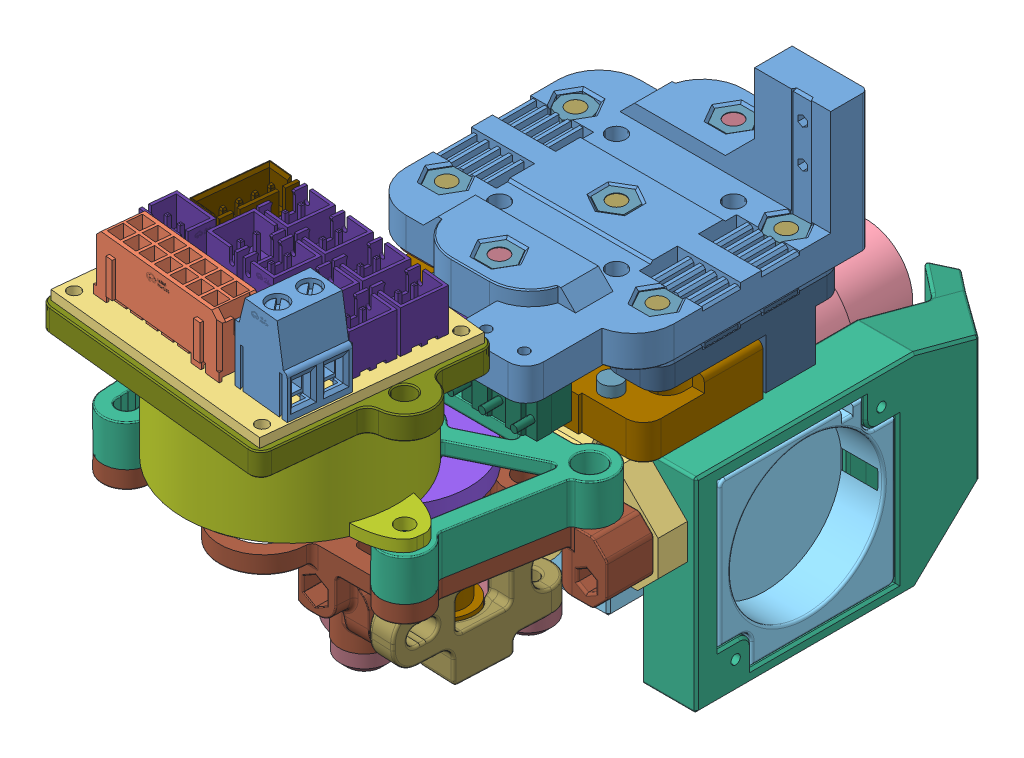
SolidWorks assembly TAP+换头组装, configuration 默认. Lengths in mm.
Overall size (64.42 74.4 119.93).
93 component instances, 36 part files, 59 mates.
Components (placement in the parent):
- TAP+换头-底座-1: TAP+换头-底座 [默认] at (-24.6795 -3.9341 35) size (46 23.5 58)
- MGN9H v1 v1-1: MGN9H v1 v1 [默认] at (-185.6361 139.1341 -146.0548) x (0 -1 0) z (-1 0 0) size (8 40.67 20)
- TAP+换头-热端装配-1: TAP+换头-热端装配 [默认] at (-3.9804 -84.1007 64.8164) x (-1 0 0) z (0 1 0) size (64.42 119.93 74.4)
  - TAP+换头-V6固定座-1: TAP+换头-V6固定座 [Default] at (0.6992 -1.423 53.775) size (52 19.4 22.55)
  - V6散热器-1: V6散热器 [Default] at (0.6992 1.577 53.775) x (-0.937959 0 -0.346747) z (-0.346747 0 0.937959) size (22.3 59 22.3)
  - TAP+换头-V6固定座-1-1: TAP+换头-V6固定座-1 [Default] at (0.6992 -1.423 53.775) x (-1 0 0) z (0 0 -1) size (35 25.4 12.09)
  - 挤出机组装-1: 挤出机组装 [Default] at (24.2197 76.008 94.8824) x (-1 0 0) z (0 -1 0) size (60.01 46.35 49.65)
    - 挤出机电机座-1: 挤出机电机座 [Default] at (-24.1653 27.1074 25.8748) size (56.72 7.01 44.47)
    - 36圆饼电机-1: 36圆饼电机 [Default] at (15.4671 9.6074 38.1257) x (0.994716 0 -0.102664) z (0.102664 0 0.994716) size (49.93 29 36.4)
    - BMG主齿组装-1: BMG主齿组装 [Default] at (16.3112 26.812 26.7681) x (0.995449 0 0.095298) z (-0.095298 0 0.995449) size (25.9 28.3 25.9)
      - BMG主齿-1: BMG主齿 [Default] at (5.4147 0.2954 24.6592) size (25.9 28.3 25.9)
      - BMG挤出齿-1: BMG挤出齿 [Default] at (5.4147 25.5954 24.6592) x (-0.887226 0 -0.461335) z (-0.461335 0 0.887226) size (9.4 14 9.4)
    - MR85-1: MR85 [Default] at (19.3513 27.6074 51.831) size (8 2.5 8)
    - 挤出机主体-1: 挤出机主体 [Default] at (-24.1653 34.1074 25.8748) size (59.44 18.3 40.97)
    - 挤出机从挤出齿轮支架-1: 挤出机从挤出齿轮支架 [Default] at (34.3823 55.9074 36.7653) x (0.043131 0 0.999069) z (0 -1 0) size (30 8.53 21.09)
    - BMG挤出齿-2: BMG挤出齿 [Default] at (28.0327 52.4074 51.9833) x (-0.837169 0 -0.546944) z (-0.546944 0 0.837169) size (9.4 14 9.4)
    - 挤出机盖子-1: 挤出机盖子 [Default] at (19.3513 55.9074 51.831) x (0.999977 0 0.006798) z (0.006798 0 -0.999977) size (25.23 3.5 27.46)
    - MR85-2: MR85 [Default] at (19.3513 54.9074 51.831) x (-0.837169 0 -0.546944) z (-0.546944 0 0.837169) size (8 2.5 8)
  - M3螺母-1: M3螺母 [默认] at (12.1907 1.0199 62.875) x (-0.783317 0.621622 0) z (0.621622 0.783317 0) size (6.35 2.3 5.5)
  - M3x20-1: M3x20 [Default] at (12.1992 1.077 65.275) x (-0.825766 -0.564012 0) z (0 0 -1) size (5.7 5.7 23)
  - M3螺母-2: M3螺母 [默认] at (-10.8461 1.0411 62.875) x (-0.929999 0.367561 0) z (0.367561 0.929999 0) size (6.35 2.3 5.5)
  - M3x20-2: M3x20 [Default] at (-10.8461 1.0411 65.275) x (-0.518434 0.855118 0) z (0 0 -1) size (5.7 5.7 23)
  - PCB固定-2-2: PCB固定-2 [默认] at (-13.6764 25.1175 89.275) x (0.102664 0.994716 0) z (-0.994716 0.102664 0) size (37 4 53.35)
  - 3D_HeadBoard_2024-03-10.step-1: 3D_HeadBoard_2024-03-10.step [默认] at (-8.9858 60.8247 89.275) x (0.994716 -0.102664 0) z (0 0 1) size (39.97 34.97 17.5)
    - FAN2.step-1: FAN2.step [默认] at (13.0535 -19.558 1.6001) x (0 -1 0) z (0 0 1) size (7.5 5.9 10.6)
      - CONN-TH_2P-P2.50_HX25003-2A.step-1: CONN-TH_2P-P2.50_HX25003-2A.step [默认] at origin size (7.5 5.9 10.6)
        - COMPOUND.step-1: COMPOUND.step [默认] at origin size (7.5 5.9 10.6)
    - PROBE.step-1: PROBE.step [默认] at (13.0535 -27.5591 1.6001) x (0 -1 0) z (0 0 1) size (7.5 5.9 10.6)
      - CONN-TH_2P-P2.50_HX25003-2A.step-1: CONN-TH_2P-P2.50_HX25003-2A.step [默认] at origin size (7.5 5.9 10.6)
        - COMPOUND.step-1: COMPOUND.step [默认] at origin size (7.5 5.9 10.6)
    - TEM1.step-1: TEM1.step [默认] at (27.4766 -27.5591 1.6001) x (0 -1 0) z (0 0 1) size (7.5 5.9 10.6)
      - CONN-TH_2P-P2.50_HX25003-2A.step-1: CONN-TH_2P-P2.50_HX25003-2A.step [默认] at origin size (7.5 5.9 10.6)
        - COMPOUND.step-1: COMPOUND.step [默认] at origin size (7.5 5.9 10.6)
    - TEM2.step-1: TEM2.step [默认] at (20.2651 -27.5591 1.6001) x (0 -1 0) z (0 0 1) size (7.5 5.9 10.6)
      - CONN-TH_2P-P2.50_HX25003-2A.step-1: CONN-TH_2P-P2.50_HX25003-2A.step [默认] at origin size (7.5 5.9 10.6)
        - COMPOUND.step-1: COMPOUND.step [默认] at origin size (7.5 5.9 10.6)
    - 5V.step-1: 5V.step [默认] at (34.6711 -14.859 1.6001) size (7.5 5.9 10.6)
      - CONN-TH_2P-P2.50_HX25003-2A.step-1: CONN-TH_2P-P2.50_HX25003-2A.step [默认] at origin size (7.5 5.9 10.6)
        - COMPOUND.step-1: COMPOUND.step [默认] at origin size (7.5 5.9 10.6)
    - FAN2-1.step-1: FAN2-1.step [默认] at (5.842 -19.558 1.6001) x (0 -1 0) z (0 0 1) size (7.5 5.9 10.6)
      - CONN-TH_2P-P2.50_HX25003-2A.step-1: CONN-TH_2P-P2.50_HX25003-2A.step [默认] at origin size (7.5 5.9 10.6)
        - COMPOUND.step-1: COMPOUND.step [默认] at origin size (7.5 5.9 10.6)
    - X-ENDSTOP.step-1: X-ENDSTOP.step [默认] at (5.842 -27.5591 1.6001) x (0 -1 0) z (0 0 1) size (7.5 5.9 10.6)
      - CONN-TH_2P-P2.50_HX25003-2A.step-1: CONN-TH_2P-P2.50_HX25003-2A.step [默认] at origin size (7.5 5.9 10.6)
        - COMPOUND.step-1: COMPOUND.step [默认] at origin size (7.5 5.9 10.6)
    - VCC.step-1: VCC.step [默认] at (26.1621 -19.558 1.6001) x (0 1 0) z (0 0 1) size (7.5 5.9 10.6)
      - CONN-TH_2P-P2.50_HX25003-2A.step-1: CONN-TH_2P-P2.50_HX25003-2A.step [默认] at origin size (7.5 5.9 10.6)
        - COMPOUND.step-1: COMPOUND.step [默认] at origin size (7.5 5.9 10.6)
    - FAN1.step-1: FAN1.step [默认] at (20.2651 -19.558 1.6001) x (0 -1 0) z (0 0 1) size (7.5 5.9 10.6)
      - CONN-TH_2P-P2.50_HX25003-2A.step-1: CONN-TH_2P-P2.50_HX25003-2A.step [默认] at origin size (7.5 5.9 10.6)
        - COMPOUND.step-1: COMPOUND.step [默认] at origin size (7.5 5.9 10.6)
    - E_MOTO.step-1: E_MOTO.step [默认] at (33.2741 -25.0864 1.6001) x (0 -1 0) z (0 0 1) size (12.5 5.7 10)
      - CONN-TH_4P-P2.50_4PIN.step-1: CONN-TH_4P-P2.50_4PIN.step [默认] at origin size (12.5 5.7 10)
        - COMPOUND-0.step-1: COMPOUND-0.step [默认] at origin size (12.5 5.7 10)
    - HOT.step-1: HOT.step [默认] at (5.842 -9.652 1.6001) x (0 1 0) z (0 0 1) size (10.76 10 17.5)
      - CONN-TH_2P-P5.00_WJ500V-5.08-2P.step-1: CONN-TH_2P-P5.00_WJ500V-5.08-2P.step [默认] at origin size (10.76 10 17.5)
        - COMPOUND-1.step-1: COMPOUND-1.step [默认] at origin size (10.76 10 17.5)
    - HEAD_IN.step-1: HEAD_IN.step [默认] at (24.003 -6.858 1.6001) x (-1 0 0) z (0 0 1) size (24 8.8 13.2)
      - CONN-TH_14P-P3.00_HC-MX3.0-2X7A.step-1: CONN-TH_14P-P3.00_HC-MX3.0-2X7A.step [默认] at origin size (24 8.8 13.2)
        - SOLID.step-1: SOLID.step [默认] at origin size (24 8.8 13.2)
    - COMPOUND-2.step-1: COMPOUND-2.step [默认] at origin size (39.97 34.97 1.6)
  - 3010风扇-1: 3010风扇 [Default] at (-14.3008 -39.823 42.275) x (1 0 0) z (0 1 0) size (30 10 30)
  - 3010涡轮-1: 3010涡轮 [Default] at (-16.8008 0.077 32.875) x (0 0 1) z (0 -1 0) size (30 10.07 30)
  - V2吹料-1-1: V2吹料-1 [默认] at (-26.8008 0.077 65.275) size (16.15 60.54 34.8)
  - 镜向V2吹料-1-2: 镜向V2吹料-1 [默认] at (28.1992 0.077 65.275) x (-1 0 0) z (0 0 -1) size (16.15 60.54 34.8)
  - 3010涡轮-2: 3010涡轮 [Default] at (18.1992 0.077 62.875) x (0 0 -1) z (0 -1 0) size (30 10.07 30)
- MGN9-6-1: MGN9-6 [默认] at (-4.6795 -6.5841 292.5) x (1 0 0) z (0 0 -1) size (9 6.5 50)
- TAP+换头中间座-1: TAP+换头中间座 [默认] at (-17.1795 -17.3341 73.9934) size (46 8.6 30)
- TAP+换头皮带盖板-2: TAP+换头皮带盖板 [默认] at (8.3205 -7.9341 71) size (10 12.6 32)
- TAP+换头皮带盖板-2-1: TAP+换头皮带盖板-2 [默认] at (-27.6795 -7.9341 71) size (10 12.6 32)
- M3x8-1: M3x8 [Default] at (-22.6795 1.0659 66) x (0.99943 0 -0.033759) z (0 -1 0) size (5.7 5.7 11)
- M3x8-2: M3x8 [Default] at (-22.6795 1.0659 44) x (0.753968 0 0.656911) z (0 -1 0) size (5.7 5.7 11)
- M3x8-4: M3x8 [Default] at (13.3205 1.0659 66) x (0.058047 0 -0.998314) z (0 -1 0) size (5.7 5.7 11)
- M3x8-5: M3x8 [Default] at (13.3205 1.0659 44) x (0.586032 0 0.810288) z (0 -1 0) size (5.7 5.7 11)
- M3x8-7: M3x8 [Default] at (-4.6795 1.6659 54.992) x (-0.906074 0 -0.423119) z (0 -1 0) size (5.7 5.7 11)
- M3螺母-2: M3螺母 [默认] at (13.3205 -1.2341 66) x (0.512033 0 -0.858966) z (0.858966 0 0.512033) size (6.35 2.3 5.5)
- M3螺母-3: M3螺母 [默认] at (-4.6795 -0.5341 55) x (-0.011209 0 -0.999937) z (0.999937 0 -0.011209) size (6.35 2.3 5.5)
- M3螺母-4: M3螺母 [默认] at (-4.6795 1.4659 75) size (6.35 2.3 5.5)
- M3x10-2: M3x10 [Default] at (-4.6795 3.6659 75) x (-0.258789 0 0.965934) z (0 -1 0) size (5.7 5.7 13)
- M3螺母-5: M3螺母 [默认] at (-4.6795 1.4659 35) size (6.35 2.3 5.5)
- M3x10-3: M3x10 [Default] at (-4.6795 3.6659 35) x (-0.379423 0 -0.925223) z (0 -1 0) size (5.7 5.7 13)
- M3螺母-6: M3螺母 [默认] at (13.3205 -1.2341 44) x (0.999299 0 -0.037424) z (0.037424 0 0.999299) size (6.35 2.3 5.5)
- M3螺母-7: M3螺母 [默认] at (-22.6795 -1.2341 66) size (6.35 2.3 5.5)
- M3螺母-8: M3螺母 [默认] at (-22.6795 -1.2341 44) x (0.719334 0 -0.694664) z (0.694664 0 0.719334) size (6.35 2.3 5.5)
- M2x8-1: M2x8 [Default] at (-17.1795 -18.2341 58.9934) x (-0.826538 0 -0.562881) z (0 1 0) size (3.6 3.6 9.8)
- M2x8-2: M2x8 [Default] at (7.8205 -18.2341 58.9934) x (1 0 0) z (0 1 0) size (3.6 3.6 9.8)
- M2x8-3: M2x8 [Default] at (9.8205 -19.3341 70.3934) x (-0.826538 0 -0.562881) z (0 1 0) size (3.6 3.6 9.8)
- M2x8-4: M2x8 [Default] at (-19.1795 -19.3341 70.3934) x (-0.826538 0 -0.562881) z (0 1 0) size (3.6 3.6 9.8)
- KW10 Microswitch v1-1: KW10 Microswitch v1 [默认] at (86.3205 84.1659 86.4) x (1 0 0) z (0 0 -1) size (13.18 11.3 12.93)
  - M2x10 Self-tapping Screw (14) v1^KW10 Microswitch v1-1: M2x10 Self-tapping Screw (14) v1^KW10 Microswitch v1 [默认] at (-76.75 95.2 1.4) x (0 0 1) z (0 1 0) size (3.5 3.5 11.3) (hidden, virtual)
  - M2x10 Self-tapping Screw (14) v1 (1)^KW10 Microswitch v1-1: M2x10 Self-tapping Screw (14) v1 (1)^KW10 Microswitch v1 [默认] at (-83.25 95.2 1.4) x (0 0 1) z (0 1 0) size (3.5 3.5 11.3) (hidden, virtual)
  - KW10 Microswitch v1-3^KW10 Microswitch v1-1: KW10 Microswitch v1-3^KW10 Microswitch v1 [默认] at origin size (13.08 3.8 4.39) (hidden, virtual)
  - KW10 Microswitch v1-4^KW10 Microswitch v1-1: KW10 Microswitch v1-4^KW10 Microswitch v1 [默认] at origin size (12.8 5.8 10.15) (virtual)
Mates (geometry in assembly coordinates):
- 重合4: coincident anti-aligned: plane of MGN9H v1 v1-1 through (-4.6795 -9.8341 73.9434) normal (0 1 0); plane of MGN9-6-1 through (-8.9795 -9.8341 42.5) normal (0 -1 0)
- 重合5: coincident anti-aligned: plane of MGN9H v1 v1-1 through (-9.1795 -9.3341 73.9434) normal (1 0 0); plane of MGN9-6-1 through (-9.1795 -3.5341 42.5) normal (-1 0 0)
- 同心9: concentric aligned: cylinder of MGN9H v1 v1-1 through (2.8205 -10.3341 50.9934) axis (0 -1 0) radius 1.5; cylinder of TAP+换头中间座-1 through (2.8205 -13.3341 50.9934) axis (0 -1 0) radius 1.6
- 同心10: concentric aligned: cylinder of MGN9H v1 v1-1 through (-12.1795 -10.3341 66.9934) axis (0 -1 0) radius 1.5; cylinder of TAP+换头中间座-1 through (-12.1795 -13.3341 66.9934) axis (0 -1 0) radius 1.6
- 重合10: coincident anti-aligned: plane of MGN9H v1 v1-1 through (-4.6795 -13.3341 73.9434) normal (0 -1 0); plane of TAP+换头中间座-1 through (-17.1795 -13.3341 73.9934) normal (0 1 0)
- 同心21: concentric anti-aligned: cylinder of TAP+换头中间座-1 through (13.3205 -12.5341 55.7934) axis (0 0 -1) radius 3.15; cylinder of TAP+换头皮带盖板-2 through (13.3205 -12.5341 49.7) axis (0 0 1) radius 3.15
- 同心26: concentric anti-aligned: cylinder of MGN9-6-1 through (-4.6795 -9.8341 35) axis (0 1 0) radius 1.7; cylinder of TAP+换头-底座-1 through (-4.6795 1.9659 35) axis (0 -1 0) radius 1.6
- 同心27: concentric anti-aligned: cylinder of MGN9-6-1 through (-4.6795 -9.8341 75) axis (0 1 0) radius 1.7; cylinder of TAP+换头-底座-1 through (-4.6795 1.9659 75) axis (0 -1 0) radius 1.6
- 重合24: coincident anti-aligned: plane of MGN9-6-1 through (-8.9795 -3.3341 42.5) normal (0 1 0); plane of TAP+换头-底座-1 through (-24.6795 -3.3341 35) normal (0 -1 0)
- 平行6: parallel aligned: plane of MGN9-6-1 through (-11.0442 1.6478 80) normal (0 0 1); plane of TAP+换头-热端装配-1/TAP+换头-V6固定座-1-1 through (-4.6795 -30.3257 73.8934) normal (0 0 1)
- 同心33: concentric anti-aligned: cylinder of TAP+换头-热端装配-1/TAP+换头-V6固定座-1 through (-17.1795 -19.8257 58.9934) axis (0 1 0) radius 1.95; cylinder of TAP+换头中间座-1 through (-17.1795 -8.7341 58.9934) axis (0 -1 0) radius 1.1
- 同心34: concentric anti-aligned: cylinder of TAP+换头-热端装配-1/TAP+换头-V6固定座-1 through (7.8205 -19.8257 58.9934) axis (0 1 0) radius 1.95; cylinder of TAP+换头中间座-1 through (7.8205 -8.7341 58.9934) axis (0 -1 0) radius 1.1
- 同心36: concentric anti-aligned: cylinder of TAP+换头皮带盖板-2 through (13.3205 -3.9341 44) axis (0 -1 0) radius 1.6; cylinder of TAP+换头-底座-1 through (13.3205 -8.4341 44) axis (0 1 0) radius 1.6
- 同心37: concentric anti-aligned: cylinder of TAP+换头皮带盖板-2 through (13.3205 -3.9341 66) axis (0 -1 0) radius 1.6; cylinder of TAP+换头-底座-1 through (13.3205 -8.4341 66) axis (0 1 0) radius 1.6
- 同心46: concentric anti-aligned: cylinder of TAP+换头-底座-1 through (-22.6795 -8.4341 66) axis (0 1 0) radius 1.6; cylinder of TAP+换头皮带盖板-2-1 through (-22.6795 -3.9341 66) axis (0 -1 0) radius 1.6
- 同心47: concentric anti-aligned: cylinder of TAP+换头-底座-1 through (-22.6795 -8.4341 44) axis (0 1 0) radius 1.6; cylinder of TAP+换头皮带盖板-2-1 through (-22.6795 -3.9341 44) axis (0 -1 0) radius 1.6
- 重合58: coincident anti-aligned: plane of TAP+换头-底座-1 through (-24.6795 -3.9341 35) normal (0 -1 0); plane of TAP+换头皮带盖板-2-1 through (-27.6795 -3.9341 71) normal (0 1 0)
- 同心53: concentric anti-aligned: cylinder of TAP+换头中间座-1 through (-4.6795 -15.2341 62.9934) axis (0 -1 0) radius 4.25; cylinder of TAP+换头-热端装配-1/TAP+换头-V6固定座-1 through (-4.6795 -20.9257 62.9934) axis (0 1 0) radius 4.25
- 同心54: concentric anti-aligned: cylinder of TAP+换头皮带盖板-2-1 through (-22.6795 -6.9341 66) axis (0 -1 0) radius 3; cylinder of M3x8-1 through (-22.6795 -6.9341 66) axis (0 1 0) radius 1.5
- 重合72: coincident anti-aligned: plane of TAP+换头皮带盖板-2-1 through (-22.6795 -6.9341 66) normal (0 -1 0); plane of M3x8-1 through (-22.6795 -6.9341 66) normal (0 1 0)
- 同心55: concentric aligned: cylinder of TAP+换头皮带盖板-2-1 through (-22.6795 -16.5341 44) axis (0 1 0) radius 3; cylinder of M3x8-2 through (-22.6795 -9.9341 44) axis (0 1 0) radius 2.85
- 重合73: coincident aligned: plane of TAP+换头皮带盖板-2-1 through (-22.6795 -6.9341 44) normal (0 -1 0); circle of M3x8-2
- 同心56: concentric anti-aligned: circle of TAP+换头皮带盖板-2; cylinder of M3x8-4 through (13.3205 -6.9341 66) axis (0 1 0) radius 1.5
- 重合74: coincident anti-aligned: plane of TAP+换头皮带盖板-2 through (13.3205 -6.9341 66) normal (0 -1 0); plane of M3x8-4 through (13.3205 -6.9341 66) normal (0 1 0)
- 同心57: concentric anti-aligned: cylinder of TAP+换头皮带盖板-2 through (13.3205 -3.9341 44) axis (0 -1 0) radius 1.6; cylinder of M3x8-5 through (13.3205 -6.9341 44) axis (0 1 0) radius 1.5
- 重合75: coincident anti-aligned: plane of TAP+换头皮带盖板-2 through (13.3205 -6.9341 44) normal (0 -1 0); plane of M3x8-5 through (13.3205 -6.9341 44) normal (0 1 0)
- 重合81: coincident anti-aligned: plane of MGN9-6-1 through (-4.6795 -6.3341 75) normal (0 -1 0); plane of M3x8-7 through (-4.6795 -6.3341 54.992) normal (0 1 0)
- 重合82: coincident anti-aligned: plane of TAP+换头-底座-1 through (-24.6795 -1.2341 35) normal (0 1 0); plane of M3螺母-2 through (13.3205 -1.2341 66) normal (0 -1 0)
- 同心62: concentric aligned: circle of TAP+换头-底座-1; cylinder of M3螺母-2 through (13.3205 1.0659 66) axis (0 -1 0) radius 1.5
- 同心63: concentric aligned: cylinder of TAP+换头-底座-1 through (-4.6795 1.9659 55) axis (0 -1 0) radius 1.6; cylinder of M3螺母-3 through (-4.6795 1.7659 55) axis (0 -1 0) radius 1.5
- 重合83: coincident anti-aligned: plane of TAP+换头-底座-1 through (-24.6795 -0.5341 35) normal (0 1 0); plane of M3螺母-3 through (-4.6795 -0.5341 55) normal (0 -1 0)
- 平行10: parallel anti-aligned: plane of TAP+换头-底座-1 through (-4.7158 -0.5341 51.767) normal (0.509676 0 0.860366); plane of M3螺母-3 through (-4.7151 1.7659 51.8248) normal (-0.509676 0 -0.860366)
- 同心64: concentric aligned: circle of TAP+换头-底座-1; cylinder of M3螺母-4 through (-4.6795 3.7659 75) axis (0 -1 0) radius 1.5
- 重合87: coincident anti-aligned: plane of TAP+换头-底座-1 through (-24.6795 1.4659 35) normal (0 1 0); plane of M3螺母-4 through (-4.6795 1.4659 75) normal (0 -1 0)
- 同心66: concentric aligned: cylinder of MGN9-6-1 through (-4.6795 -8.3341 54.992) axis (0 1 0) radius 3; cylinder of M3x8-7 through (-4.6795 -6.3341 54.992) axis (0 1 0) radius 1.5
- 同心67: concentric aligned: cylinder of MGN9-6-1 through (-4.6795 -9.8341 75) axis (0 1 0) radius 1.7; cylinder of M3x10-2 through (-4.6795 -6.3341 75) axis (0 1 0) radius 1.5
- 重合89: coincident aligned: plane of M3x8-7 through (-4.6795 -9.3341 54.992) normal (0 -1 0); plane of M3x10-2 through (-4.6795 -9.3341 75) normal (0 -1 0)
- 重合90: coincident anti-aligned: plane of TAP+换头-底座-1 through (-24.6795 1.4659 35) normal (0 1 0); plane of M3螺母-5 through (-4.6795 1.4659 35) normal (0 -1 0)
- 同心68: concentric aligned: cylinder of TAP+换头-底座-1 through (-4.6795 1.9659 35) axis (0 -1 0) radius 1.6; cylinder of M3螺母-5 through (-4.6795 3.7659 35) axis (0 -1 0) radius 1.5
- 同心69: concentric aligned: cylinder of MGN9-6-1 through (-4.6795 -9.8341 35) axis (0 1 0) radius 1.7; cylinder of M3x10-3 through (-4.6795 -6.3341 35) axis (0 1 0) radius 1.5
- 重合91: coincident aligned: plane of M3x8-7 through (-4.6795 -9.3341 54.992) normal (0 -1 0); plane of M3x10-3 through (-4.6795 -9.3341 35) normal (0 -1 0)
- 同心70: concentric anti-aligned: cylinder of M3x8-5 through (13.3205 -6.9341 44) axis (0 1 0) radius 1.5; cylinder of M3螺母-6 through (13.3205 1.0659 44) axis (0 -1 0) radius 1.5
- 重合93: coincident anti-aligned: plane of TAP+换头-底座-1 through (-24.6795 -1.2341 35) normal (0 1 0); plane of M3螺母-6 through (13.3205 -1.2341 44) normal (0 -1 0)
- 同心71: concentric anti-aligned: cylinder of M3x8-2 through (-22.6795 -6.9341 44) axis (0 1 0) radius 1.5; cylinder of M3螺母-8 through (-22.6795 1.0659 44) axis (0 -1 0) radius 1.5
- 重合94: coincident anti-aligned: plane of TAP+换头-底座-1 through (-24.6795 -1.2341 35) normal (0 1 0); plane of M3螺母-8 through (-22.6795 -1.2341 44) normal (0 -1 0)
- 重合95: coincident anti-aligned: plane of TAP+换头-底座-1 through (-24.6795 -1.2341 35) normal (0 1 0); plane of M3螺母-7 through (-22.6795 -1.2341 66) normal (0 -1 0)
- 重合96: coincident aligned: circle of M3x8-1; cylinder of M3螺母-7 through (-22.6795 1.0659 66) axis (0 -1 0) radius 1.5
- 同心80: concentric aligned: cylinder of TAP+换头中间座-1 through (-17.1795 -8.7341 58.9934) axis (0 -1 0) radius 1.1; cylinder of M2x8-1 through (-17.1795 -10.2341 58.9934) axis (0 -1 0) radius 1
- 重合111: coincident anti-aligned: plane of TAP+换头中间座-1 through (-17.1795 -10.2341 58.9934) normal (0 1 0); plane of M2x8-1 through (-17.1795 -10.2341 58.9934) normal (0 -1 0)
- 同心81: concentric anti-aligned: cylinder of TAP+换头中间座-1 through (7.8205 -10.2341 58.9934) axis (0 1 0) radius 2; cylinder of M2x8-2 through (7.8205 -10.2341 58.9934) axis (0 -1 0) radius 1
- 重合112: coincident anti-aligned: plane of TAP+换头中间座-1 through (7.8205 -10.2341 58.9934) normal (0 1 0); plane of M2x8-2 through (7.8205 -10.2341 58.9934) normal (0 -1 0)
- 同心82: concentric aligned: cylinder of TAP+换头中间座-1 through (-19.1795 -10.9341 70.3934) axis (0 -1 0) radius 1.05; cylinder of M2x8-4 through (-19.1795 -11.3341 70.3934) axis (0 -1 0) radius 1
- 重合113: coincident anti-aligned: plane of TAP+换头中间座-1 through (-17.1795 -11.3341 73.9934) normal (0 1 0); plane of M2x8-4 through (-19.1795 -11.3341 70.3934) normal (0 -1 0)
- 同心83: concentric aligned: cylinder of TAP+换头中间座-1 through (9.8205 -10.9341 70.3934) axis (0 -1 0) radius 1.05; cylinder of M2x8-3 through (9.8205 -11.3341 70.3934) axis (0 -1 0) radius 1
- 重合114: coincident anti-aligned: plane of TAP+换头中间座-1 through (-17.1795 -11.3341 73.9934) normal (0 1 0); plane of M2x8-3 through (9.8205 -11.3341 70.3934) normal (0 -1 0)
- 重合119: coincident anti-aligned: plane of MGN9-6-1 through (-11.0442 1.6478 80) normal (0 0 1); plane of KW10 Microswitch v1-1/KW10 Microswitch v1-4^KW10 Microswitch v1-1 through (6.3205 -6.8341 80) normal (0 0 -1)
- 重合120: coincident anti-aligned: plane of TAP+换头-底座-1 through (-24.6795 -3.9341 35) normal (0 -1 0); plane of KW10 Microswitch v1-1/KW10 Microswitch v1-4^KW10 Microswitch v1-1 through (-0.0795 -3.9341 86.5) normal (0 1 0)
- 同心84: concentric aligned: cylinder of TAP+换头-底座-1 through (9.5705 19.9507 85) axis (0 -1 0) radius 0.85; cylinder of KW10 Microswitch v1-1/KW10 Microswitch v1-4^KW10 Microswitch v1-1 through (9.5705 -3.9341 85) axis (0 -1 0) radius 1
- 同心85: concentric aligned: cylinder of TAP+换头-底座-1 through (3.0705 19.9507 85) axis (0 -1 0) radius 0.85; cylinder of KW10 Microswitch v1-1/KW10 Microswitch v1-4^KW10 Microswitch v1-1 through (3.0705 -3.9341 85) axis (0 -1 0) radius 1.2
